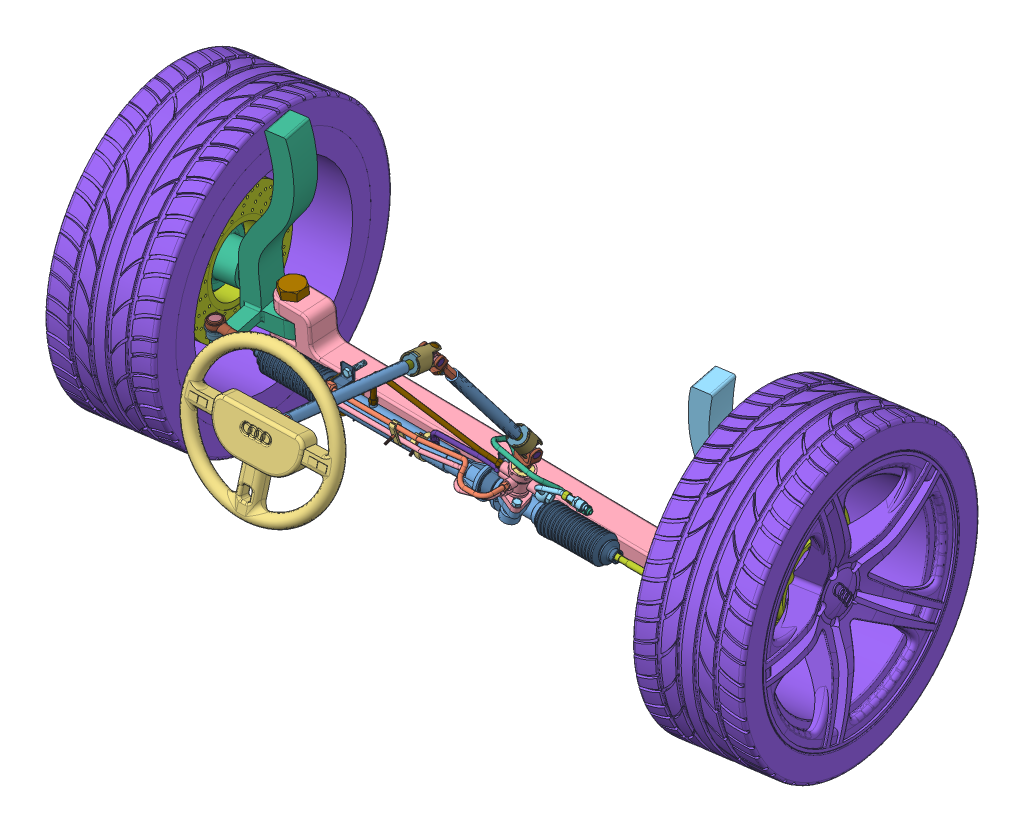
SolidWorks assembly 07, configuration Varsayılan. Lengths in mm.
Overall size (1849.54 1285.36 1549.53).
115 component instances, 65 part files, 142 mates.
Components (placement in the parent):
- 04-04-1: 04-04 [Varsayılan] at (-125.6681 -6.1583 231.0307) size (234.82 71.44 100.51)
- 04-02-1: 04-02 [Varsayılan] at (209.0718 -6.1583 231.0307) x (0 -1 0) z (-1 0 0) size (38 38 598)
- 04-03-1: 04-03 [Varsayılan] at (38.6922 -33.6461 251.0307) x (-0.603132 0.16779 0.779794) z (-0.75128 0.208941 -0.626037) size (25.52 151.51 25.52)
- 04-01-1: 04-01 [Varsayılan] at (50.1654 -6.1583 196.9106) x (0 0 1) z (-1 0 0) size (4.12 38.49 38.49)
- 04-05-1: 04-05 [Varsayılan] at (50.1654 -6.1583 220.9669) x (0 0 1) z (-1 0 0) size (15.7 26.77 26.77)
- 04-06-1: 04-06 [Varsayılan] at (50.1654 -6.1583 203.9669) x (-1 0 0) z (0 0 -1) size (18.46 18.46 19.47)
- 04-07-1: 04-07 [Varsayılan] at (50.1654 -6.1583 223.256) x (0 0 1) z (-1 0 0) size (13.68 21.45 8.13)
- 04-08-1: 04-08 [Varsayılan] at (50.1654 -6.1583 218.4607) x (0 1 0) z (-1 0 0) size (28.57 26.12 28.57)
- 05-14-1: 05-14 [Varsayılan] at (37.0194 -39.6612 251.0307) x (0.963448 -0.267897 0) z (0 0 1) size (30.59 16.59 30.59)
- 05-15-1: 05-15 [Varsayılan] at (41.4642 -23.6793 251.0307) x (0.963434 -0.267944 0) z (0 0 1) size (27.84 7.6 27.84)
- 05-21-1: 05-21 [Varsayılan] at (38.6909 -33.6508 251.0307) x (0.928206 -0.258147 -0.267944) z (0.267944 0.963434 0) size (19.84 10.08 10.35)
- 05-09-1: 05-09 [Varsayılan] at (52.7201 16.7932 251.0307) x (0.963434 -0.267944 0) z (0 0 1) size (31.93 8.54 31.93)
- 05-24-1: 05-24 [Varsayılan] at (55.0081 25.02 251.0307) x (0.963434 -0.267944 0) z (0 0 1) size (34.48 1.46 34.48)
- 05-19-1: 05-19 [Varsayılan] at (66.8414 67.5685 251.0307) x (0.963434 -0.267944 0) z (0 0 1) size (24.62 1.21 24.62)
- 05-10-1: 05-10 [Varsayılan] at (57.7931 35.0339 251.0307) x (0.959223 -0.266824 -0.093253) z (0.089843 -0.024987 0.995642) size (34.48 33.93 34.48)
- 05-11-1: 05-11 [Varsayılan] at (60.4905 44.7327 251.0307) x (0.963421 -0.267991 0) z (0 0 1) size (34.47 2.04 34.47)
- 05-11-2: 05-11 [Varsayılan] at (62.3958 51.5835 251.0307) x (0.963421 -0.267991 0) z (0 0 1) size (34.47 2.04 34.47)
- 05-11-3: 05-11 [Varsayılan] at (64.317 58.4914 251.0307) x (0.963421 -0.267991 0) z (0 0 1) size (34.47 2.04 34.47)
- 05-11-4: 05-11 [Varsayılan] at (66.126 64.9963 251.0307) x (0.963421 -0.267991 0) z (0 0 1) size (34.47 2.04 34.47)
- 05-12-1: 05-12 [Varsayılan] at (67.6163 70.3549 251.0307) x (0.92973 -0.25852 0.26224) z (-0.252651 0.070266 0.965003) size (31.17 6.94 31.17)
- 05-13-1: 05-13 [Varsayılan] at (69.4753 77.0389 251.0307) x (0.963448 -0.267897 0) z (0 0 1) size (29.11 4.72 29.11)
- 05-16-1: 05-16 [Varsayılan] at (67.6164 70.3551 251.0307) x (0.963448 -0.267897 0) z (0 0 1) size (40.01 14.09 40.01)
- 05-22-3: 05-22 [Varsayılan] at (69.4711 77.0238 251.0307) x (0.963434 -0.267944 0) z (0 0 1) size (37.74 2.78 37.74)
- 05-18-1: 05-18 [Varsayılan] at (71.3908 83.9265 251.0307) x (0.96127 -0.267342 0.066993) z (-0.064543 0.01795 0.997753) size (40.8 2.9 40.8)
- 05-25-1: 05-25 [Varsayılan] at (57.2884 33.5525 251.0071) x (0.003637 -0.001047 -0.999993) z (0.963428 -0.267942 0.003784) size (68.03 67.23 77.18)
- formed hex screw_am-1: formed hex screw_am [B18.2.3.2M - Formed hex screw, M10 x 1.5 x 25 --25WS] at (82.3436 33.466 275.1353) x (-0.267944 -0.963434 0) z (0 0 1) size (31.63 18.48 16)
- formed hex screw_am-2: formed hex screw_am [B18.2.3.2M - Formed hex screw, M10 x 1.5 x 25 --25WS] at (36.0727 46.3346 226.9262) x (-0.267944 -0.963434 0) z (0 0 1) size (31.63 18.48 16)
- ROT MİLİ-1: ROT MİLİ [Varsayılan] at (-398.6897 77.9473 255.0381) x (1 0 0) z (0 0.086009 -0.996294) size (284.47 41.76 37.89)
  - 02-02-2: 02-02 [Varsayılan] at (3.7615 85.8588 16.6847) size (48.52 36 36)
  - 02-03-3: 02-03 [Varsayılan] at (0.4735 85.8588 16.6847) x (-1 0 0) z (0 0.000479 1) size (257.66 24 24)
  - 02-01-2: 02-01 [Varsayılan] at (2.815 90.0301 15.9062) x (0.295289 -0.871295 0.391981) z (-0.068342 0.389963 0.918291) size (28 21.64 28)
- ROT MİLİ-2: ROT MİLİ [Varsayılan] at (218.8333 -67.283 293.5918) x (-1 0 0) z (0 -0.568825 -0.822459) size (284.47 41.76 37.89)
  - 02-02-2: 02-02 [Varsayılan] at (3.7615 85.8588 16.6847) size (48.52 36 36)
  - 02-03-3: 02-03 [Varsayılan] at (0.4735 85.8588 16.6847) x (-1 0 0) z (0 0.000479 1) size (257.66 24 24)
  - 02-01-2: 02-01 [Varsayılan] at (2.815 90.0301 15.9062) x (0.295289 -0.871295 0.391981) z (-0.068342 0.389963 0.918291) size (28 21.64 28)
- 05-31-1: 05-31 [Varsayılan] at (-390.0863 -6.1583 231.0307) x (0 0.999978 0.006566) z (0 0.006566 -0.999978) size (59.07 38.45 68.81)
- 05-02-1: 05-02 [Varsayılan] at (-409.0863 -6.1583 231.0307) x (-1 0 0) z (0 -0.999688 0.024965) size (174.75 66.11 66.11)
- 05-02-2: 05-02 [Varsayılan] at (105.6183 -6.1583 231.0307) size (174.75 66.11 66.11)
- ROT BAŞI-1: ROT BAŞI [Varsayılan] at (-649.4435 -11.5817 321.1285) x (1 0 0) z (0 0.087156 -0.996195) size (99.29 68.51 54.56)
  - 03-01-1: 03-01 [Default] at (-37.7726 9.1069 90.2276) size (90.23 26.88 54.56)
  - 03-02-1: 03-02 [Varsayılan] at (-32.6694 53.6205 89.5242) x (0 -1 0) z (0.136534 0 0.990635) size (58.89 20 20)
  - 03-03-1: 03-03 [Varsayılan] at (-37.7726 -12.3176 90.2276) x (0.135044 0.003215 -0.990834) z (0.99084 0 0.135044) size (26.35 4.4 26.35)
  - 03-04-1: 03-04 [Varsayılan] at (-37.7726 28.686 90.2276) x (0.880691 0 -0.473691) z (0.473691 0 0.880691) size (39.96 25.57 39.96)
  - 03-05-1: 03-05 [Varsayılan] at (-37.7726 -9.866 90.2276) size (25.83 14.98 25.83)
- ROT BAŞI-2: ROT BAŞI [Varsayılan] at (469.5871 4.146 141.36) x (-1 0 0) z (0 -0.087156 0.996195) size (99.29 68.51 54.56)
  - 03-01-1: 03-01 [Default] at (-37.7726 9.1069 90.2276) size (90.23 26.88 54.56)
  - 03-02-1: 03-02 [Varsayılan] at (-32.6694 53.6205 89.5242) x (0 -1 0) z (0.136534 0 0.990635) size (58.89 20 20)
  - 03-03-1: 03-03 [Varsayılan] at (-37.7726 -12.3176 90.2276) x (0.135044 0.003215 -0.990834) z (0.99084 0 0.135044) size (26.35 4.4 26.35)
  - 03-04-1: 03-04 [Varsayılan] at (-37.7726 28.686 90.2276) x (0.880691 0 -0.473691) z (0.473691 0 0.880691) size (39.96 25.57 39.96)
  - 03-05-1: 03-05 [Varsayılan] at (-37.7726 -9.866 90.2276) size (25.83 14.98 25.83)
- 05-28-1: 05-28 [Varsayılan] at (-1.0263 -6.1583 231.0307) x (0 -0.759317 -0.650721) z (-1 0 0) size (54.92 54.94 38.56)
- 05-05-3: 05-05 [Varsayılan] at (-153.627 16.7021 236.5228) x (-0.999618 0.007048 -0.026719) z (0.027616 0.221471 -0.974776) size (188.63 58.73 20.5)
- 05-06-2: 05-06 [Varsayılan] at (-308.371 55.2453 229.576) x (-0.999565 0.002273 -0.029406) z (0.029339 -0.025305 -0.999249) size (348.36 70.43 41.18)
- 05-03-3: 05-03 [Varsayılan] at (-414.0863 -6.1583 231.0307) size (295 48.35 43.5)
- 05-33-1: 05-33 [Default] at (-156.8797 44.8002 297.1129) x (-1 0 0) z (0 0.302472 -0.953158) size (421.56 52.06 61.28)
- 05-01-1: 05-01 [Varsayılan] at (-173.5526 -6.1583 231.0307) x (-1 0 0) z (0 0.360562 -0.932735) size (14 137.7 76.92)
- 05-04-1: 05-04 [Varsayılan] at (-390.9146 51.2479 300.523) x (-0.991921 0.112405 0.058801) z (0.000453 0.46666 -0.884437) size (456.96 84.72 60.1)
- 05-08-1: 05-08 [Varsayılan] at (237.637 92.2948 265.4276) x (-0.997325 0.072053 -0.012308) z (-0.043043 -0.714977 -0.697822) size (140.05 46.48 89.04)
- 05-07-1: 05-07 [Varsayılan] at (228.5019 70.3353 246.6946) x (-0.999175 0.040461 0.003581) z (-0.026401 -0.579908 -0.814254) size (231 45.96 100.61)
- formed hex screw_am-3: formed hex screw_am [B18.2.3.2M - Formed hex screw, M12 x 1.75 x 25 --25WS] at (123.6594 37.5337 232.8376) x (-0.948079 0.263674 0.177825) z (-0.177825 -0.903067 0.390959) size (32.76 20.78 18)
- 05-27-1: 05-27 [Varsayılan] at (186.4406 76.9952 250.3773) x (0.044464 0.751851 0.657832) z (0.9987 -0.049876 -0.0105) size (45.68 8 10)
- 05-27-2: 05-27 [Varsayılan] at (196.4276 76.4964 250.2723) x (0.044464 0.751851 0.657832) z (-0.9987 0.049876 0.0105) size (45.68 8 10)
- hex screw_am-2: hex screw_am [B18.6.7M - M5 x 0.8 x 10 Indented HHMS --10S] at (191.9929 87.5632 252.0852) x (-0.024915 -0.657444 0.753091) z (-0.753091 0.507767 0.418362) size (13.8 9.24 8)
- prevailing torque hex nut_am-2: prevailing torque hex nut_am [AM-M5-S] at (191.6665 78.9507 261.9507) x (0.999646 -0.009344 0.024915) z (-0.024915 -0.657444 0.753091) size (8 9.81 5.3)
- 05-29-1: 05-29 [Default] at (-12.3188 -6.1583 205.6444) x (0 1 0) z (0 0 -1) size (108.96 30.28 55.85)
- 05-29-3: 05-29 [Default] at (-390.1285 -6.1115 206.1523) x (0 0.999914 0.013132) z (0 0.013132 -0.999914) size (108.96 30.28 55.85)
- formed hex screw_am-4: formed hex screw_am [B18.2.3.2M - Formed hex screw, M10 x 1.5 x 40 --26WS] at (-390.1268 33.0747 215.2976) x (0 0.013132 -0.999914) z (0.935126 0.354284 0.004653) size (46.63 18.48 16)
- formed hex screw_am-5: formed hex screw_am [B18.2.3.2M - Formed hex screw, M10 x 1.5 x 40 --26WS] at (-390.1268 -45.812 214.2616) x (0 0.013132 -0.999914) z (0.970956 -0.239236 -0.003142) size (46.63 18.48 16)
- formed hex screw_am-6: formed hex screw_am [B18.2.3.2M - Formed hex screw, M10 x 1.5 x 40 --26WS] at (-12.3171 -45.7489 214.2744) x (0 0 -1) z (0.991782 -0.12794 0) size (46.63 18.48 16)
- formed hex screw_am-7: formed hex screw_am [B18.2.3.2M - Formed hex screw, M10 x 1.5 x 40 --26WS] at (-12.3171 33.1445 213.7744) x (0 0 -1) z (0.999706 0.024251 0) size (46.63 18.48 16)
- UNIVERSAL MAFSAL-1: UNIVERSAL MAFSAL [Varsayılan] at (141.0332 165.171 256.4603) x (0.950533 -0.264356 0.163103) z (-0.267944 -0.963434 0) size (48.16 92.97 129.43)
  - 01-01-1: 01-01 [Varsayılan] at (-45.6055 2.036 86.4549) size (47 34.99 57.64)
  - 01-02-1: 01-02 [Varsayılan] at (-45.0363 8.2494 31.8587) x (-0.051046 -0.624854 0.779071) z (0 -0.780088 -0.62567) size (70.3 43.23 43.34)
  - 01-03-1: 01-03 [Varsayılan] at (-51.6055 -0.2661 32.8861) x (1 0 0) z (0 -0.62567 0.780088) size (36 31 16)
  - 01-04-1: 01-04 [Varsayılan] at (-42.5986 38.09 -5.3467) x (-0.998696 0.031938 -0.03982) z (-0.051046 -0.624854 0.779071) size (33.8 41.3 6)
  - 01-05-1: 01-05 [Varsayılan] at (-42.9049 34.3409 -0.6723) x (0.998255 -0.008733 0.058403) z (0.02969 -0.780692 -0.62421) size (32.2 29.4 32.2)
  - 01-06-1: 01-06 [Varsayılan] at (-44.4056 15.9701 22.2324) x (0.051046 0.624854 -0.779071) z (0.993628 0.046715 0.102572) size (75.7 17.29 17.32)
  - 01-07-1: 01-07 [Varsayılan] at (-25.3055 1.2861 40.5406) x (0 0 -1) z (1 0 0) size (16 16 15)
  - 01-08-1: 01-08 [Varsayılan] at (-45.6055 -12.5995 29.4036) x (0.792707 0.38141 -0.475544) z (0 -0.780088 -0.62567) size (16 16 15)
  - 01-07-2: 01-07 [Varsayılan] at (-65.9055 1.2861 40.5406) x (0 -0.633294 0.773912) z (-1 0 0) size (16 16 15)
  - 01-08-2: 01-08 [Varsayılan] at (-45.6055 15.1716 51.6775) x (0.990366 0.086641 -0.108024) z (0 0.780088 0.62567) size (16 16 15)
  - formed hex screw_am-1: formed hex screw_am [B18.2.3.2M - Formed hex screw, M6 x 1.0 x 35 --18WS] at (-62.5055 12.536 76.9549) x (1 0 0) z (0 0.052048 -0.998645) size (39.15 11.55 10)
  - prevailing torque hex nut_am-1: prevailing torque hex nut_am [AM-M6-S] at (-26.1555 12.536 76.9549) x (0 0.889289 0.457347) z (1 0 0) size (10.79 11.55 6.7)
- SHAFT 1-1: SHAFT 1 [Varsayılan] at (102.4 214.0531 312.2723) x (0.979633 -0.04367 -0.195992) z (0.15908 0.764397 0.624813) size (24 24 322.5)
- SHAFT 2-1: SHAFT 2 [Varsayılan] at (126.2619 328.7127 405.9942) x (-0.986743 0.10251 0.125818) z (0.15908 0.764397 0.624813) size (19 19 232)
- UNIVERSAL MAFSAL-2: UNIVERSAL MAFSAL [Varsayılan] at (218.869 550.0843 590.8605) x (0.981176 -0.192592 -0.014194) z (-0.15908 -0.764397 -0.624813) size (48.16 92.97 129.43)
  - 01-01-1: 01-01 [Varsayılan] at (-45.6055 2.036 86.4549) size (47 34.99 57.64)
  - 01-02-1: 01-02 [Varsayılan] at (-45.0363 8.2494 31.8587) x (-0.051046 -0.624854 0.779071) z (0 -0.780088 -0.62567) size (70.3 43.23 43.34)
  - 01-03-1: 01-03 [Varsayılan] at (-51.6055 -0.2661 32.8861) x (1 0 0) z (0 -0.62567 0.780088) size (36 31 16)
  - 01-04-1: 01-04 [Varsayılan] at (-42.5986 38.09 -5.3467) x (-0.998696 0.031938 -0.03982) z (-0.051046 -0.624854 0.779071) size (33.8 41.3 6)
  - 01-05-1: 01-05 [Varsayılan] at (-42.9049 34.3409 -0.6723) x (0.998255 -0.008733 0.058403) z (0.02969 -0.780692 -0.62421) size (32.2 29.4 32.2)
  - 01-06-1: 01-06 [Varsayılan] at (-44.4056 15.9701 22.2324) x (0.051046 0.624854 -0.779071) z (0.993628 0.046715 0.102572) size (75.7 17.29 17.32)
  - 01-07-1: 01-07 [Varsayılan] at (-25.3055 1.2861 40.5406) x (0 0 -1) z (1 0 0) size (16 16 15)
  - 01-08-1: 01-08 [Varsayılan] at (-45.6055 -12.5995 29.4036) x (0.792707 0.38141 -0.475544) z (0 -0.780088 -0.62567) size (16 16 15)
  - 01-07-2: 01-07 [Varsayılan] at (-65.9055 1.2861 40.5406) x (0 -0.633294 0.773912) z (-1 0 0) size (16 16 15)
  - 01-08-2: 01-08 [Varsayılan] at (-45.6055 15.1716 51.6775) x (0.990366 0.086641 -0.108024) z (0 0.780088 0.62567) size (16 16 15)
  - formed hex screw_am-1: formed hex screw_am [B18.2.3.2M - Formed hex screw, M6 x 1.0 x 35 --18WS] at (-62.5055 12.536 76.9549) x (1 0 0) z (0 0.052048 -0.998645) size (39.15 11.55 10)
  - prevailing torque hex nut_am-1: prevailing torque hex nut_am [AM-M6-S] at (-26.1555 12.536 76.9549) x (0 0.889289 0.457347) z (1 0 0) size (10.79 11.55 6.7)
- SHAFT 1-2: SHAFT 1 [Varsayılan] at (178.0086 547.047 663.7863) x (0.966904 0.207955 -0.147823) z (0.105608 0.201209 0.973839) size (24 24 322.5)
- SHAFT 2-2: SHAFT 2 [Varsayılan] at (191.7377 573.2042 790.3853) x (-0.993361 0.06628 0.094031) z (0.105608 0.201209 0.973839) size (19 19 232)
- direksiyon-1: direksiyon [Varsayılan] at (216.7667 620.8908 1021.1848) x (-0.993361 0.06628 0.094031) z (0.105608 0.201209 0.973839) size (350 350 50.57)
- ÖN DÜZEN-1: ÖN DÜZEN [Varsayılan] at (-260.8263 1115.8453 259.3364) x (-0.999881 0.001392 -0.015371) z (-0.000148 -0.996747 -0.080594) size (1834.03 1010.52 929.37)
  - DİNGİL-1: DİNGİL [Varsayılan] at (-152.2952 42.0235 1230.14) size (1171.64 67 117)
  - Tekerlek porya-bağlantı kolları  R-1: Tekerlek porya-bağlantı kolları  R [Varsayılan] at (-732.3489 82.2489 1097.7024) x (-0.988638 0.150316 0) z (0.150316 0.988638 0) size (231.48 449.46 221.1)
  - Tekerlek porya-bağlantı kolları L-1: Tekerlek porya-bağlantı kolları L [Varsayılan] at (427.7584 68.798 1097.7024) x (0.988638 -0.150316 0) z (-0.150316 -0.988638 0) size (231.48 449.46 221.1)
  - Fren diski-1: Fren diski [Varsayılan] at (509.8767 56.3125 1097.7024) x (-0.084581 -0.556299 0.826667) z (0.124261 0.817274 0.562692) size (303 56.33 303)
  - Tekerlek-1: Tekerlek [Varsayılan] at (-277.6343 176.0481 1097.7024) x (-0.084581 -0.556299 0.826667) z (0.124261 0.817274 0.562692) size (668.92 273.92 668.92)
  - Fren diski-2: Fren diski [Varsayılan] at (-814.4672 94.7344 1097.7024) x (-0.080555 -0.529817 -0.844277) z (0.126908 0.834685 -0.535906) size (303 56.33 303)
  - Tekerlek-2: Tekerlek [Varsayılan] at (-26.9562 -25.0012 1097.7024) x (-0.080555 -0.529817 -0.844277) z (0.126908 0.834685 -0.535906) size (668.92 273.92 668.92)
  - heavy hex bolt_am-2: heavy hex bolt_am [B18.2.3.6M - Heavy hex bolt M30 x 3.5 x 140 --72S] at (383.5248 75.5235 1093.39) x (0 0 1) z (-1 0 0) size (159.75 57.74 50)
  - hex nut heavy_am-2: hex nut heavy_am [B18.2.4.6M - Heavy hex nut,  M30 x 3.5 --W-S] at (383.5248 75.5235 1260.84) size (50 57.74 30.7)
  - heavy hex bolt_am-3: heavy hex bolt_am [B18.2.3.6M - Heavy hex bolt M30 x 3.5 x 140 --72S] at (-688.1152 75.5235 1093.39) x (0 0 1) z (-1 0 0) size (159.75 57.74 50)
  - hex nut heavy_am-3: hex nut heavy_am [B18.2.4.6M - Heavy hex nut,  M30 x 3.5 --W-S] at (-688.1152 75.5235 1260.84) size (50 57.74 30.7)
- 05-30-1: 05-30 [B18.2.3.2M - Formed hex screw, M5 x 0.8 x 40 --16WS] at (-179.5526 27.5361 241.8952) x (0 -0.741989 0.670412) z (-0.831659 0.372271 0.412016) size (43.65 9.24 8)
- 05-30-2: 05-30 [B18.2.3.2M - Formed hex screw, M5 x 0.8 x 40 --16WS] at (-179.5526 63.0693 290.0383) x (0 -0.309906 0.950767) z (-0.960688 -0.26396 -0.086039) size (43.65 9.24 8)
Mates (geometry in assembly coordinates):
- Eş Merkezli1: concentric aligned: cylinder of 04-04-1 through (-165.266 -6.1583 231.0307) axis (1 0 0) radius 14; cylinder of 04-02-1 through (-388.9282 -6.1583 231.0307) axis (1 0 0) radius 11.5
- Eş Merkezli2: concentric anti-aligned: cylinder of 04-04-1 through (54.1024 21.7633 251.0307) axis (0.267944 0.963434 0) radius 12.4576; line of 04-03-1 through (79.2895 112.3275 251.0307) axis (-0.267944 -0.963434 0)
- Teğet1: tangent aligned: plane of 04-04-1 through (55.5026 -19.6951 251.0307) normal (-0.267944 -0.963434 0); cone of 04-03-1 through (43.5006 -16.3571 251.0307) axis (-0.267944 -0.963434 0)
- Paralel1: parallel: plane of 04-02-1 through (46.1449 10.9835 238.0307) normal (0 0 1); line of 04-03-1 through (79.2895 112.3275 251.0307) axis (-0.267944 -0.963434 0)
- RackPinionMate1: rack pinion = 20 mm: line of 04-02-1 through (7.4299 -15.2825 238.0307) axis (-1 0 0); circle of 04-03-1
- Uzaklığı Sınırla1: limit distance = 45.2601 mm anti-aligned: plane of 04-04-1 through (-125.6681 11.3406 231.0307) normal (-1 0 0); plane of 04-02-1 through (-170.9282 -6.1583 250.0307) normal (1 0 0)
- Eş Merkezli3: concentric anti-aligned: cylinder of 04-05-1 through (50.1654 -6.1583 220.9669) axis (0 0 -1) radius 3.705; cylinder of 04-07-1 through (50.1654 -6.1583 223.256) axis (0 0 1) radius 3.7071
- Eş Merkezli4: concentric: sphere of 04-05-1; unknown of 04-07-1
- Eş Merkezli5: concentric anti-aligned: circle of 04-06-1; cylinder of 04-07-1 through (50.1654 -6.1583 223.256) axis (0 0 1) radius 3.7071
- Çakışık1: coincident anti-aligned: plane of 04-05-1 through (59.8031 -6.1583 220.9669) normal (0 0 -1); plane of 04-06-1 through (40.4527 -15.387 220.9669) normal (0 0 1)
- Eş Merkezli6: concentric anti-aligned: circle of 04-06-1; cylinder of 04-08-1 through (50.1654 -6.1583 199.3607) axis (0 0 1) radius 14.285
- Çakışık2: coincident anti-aligned: plane of 04-05-1 through (63.3694 -6.1583 218.4607) normal (0 0 -1); plane of 04-08-1 through (50.1654 -6.1583 218.4607) normal (0 0 1)
- Eş Merkezli7: concentric anti-aligned: cylinder of 04-04-1 through (50.1654 -6.1583 285.0814) axis (0 0 -1) radius 14; cylinder of 04-08-1 through (50.1654 -6.1583 199.3607) axis (0 0 1) radius 14.285
- Çakışık3: coincident anti-aligned: plane of 04-04-1 through (50.1654 -6.1583 201.0307) normal (0 0 -1); circle of 04-08-1
- Eş Merkezli8: concentric anti-aligned: cylinder of 04-04-1 through (50.1654 -6.1583 201.0307) axis (0 0 1) radius 18.85; cylinder of 04-01-1 through (50.1654 -6.1583 196.9106) axis (0 0 -1) radius 13.3852
- Çakışık4: coincident anti-aligned: plane of 04-04-1 through (50.1654 -6.1583 201.0307) normal (0 0 -1); plane of 04-01-1 through (63.5506 -6.1583 201.0307) normal (0 0 1)
- Eş Merkezli9: concentric anti-aligned: cylinder of 04-04-1 through (54.1024 21.7633 251.0307) axis (0.267944 0.963434 0) radius 15.0252; cylinder of 05-15-1 through (43.5005 -16.3572 251.0307) axis (-0.267944 -0.963434 0) radius 13.92
- Çakışık5: coincident anti-aligned: plane of 04-04-1 through (55.5026 -19.6951 251.0307) normal (-0.267944 -0.963434 0); plane of 05-15-1 through (43.5005 -16.3572 251.0307) normal (0.267944 0.963434 0)
- Eş Merkezli10: concentric aligned: cone of 04-03-1 through (38.6923 -33.6459 251.0307) axis (0.267944 0.963434 0); cylinder of 05-21-1 through (38.6909 -33.6508 251.0307) axis (0.267944 0.963434 0) radius 4.26
- Çakışık6: coincident anti-aligned: plane of 05-15-1 through (41.4642 -23.6793 251.0307) normal (-0.267944 -0.963434 0); plane of 05-21-1 through (41.4642 -23.6793 251.0307) normal (0.267944 0.963434 0)
- Eş Merkezli11: concentric aligned: cylinder of 04-04-1 through (54.1024 21.7633 251.0307) axis (0.267944 0.963434 0) radius 15.0252; cone of 05-14-1 through (39.1828 -31.8821 251.0307) axis (0.267944 0.963434 0)
- Teğet2: tangent aligned: cone of 05-14-1 through (41.4644 -23.6786 251.0307) axis (-0.267944 -0.963434 0); plane of 05-15-1 through (41.4642 -23.6793 251.0307) normal (-0.267944 -0.963434 0)
- Çakışık7: coincident: circle of 04-03-1; cylinder of 05-09-1 through (52.7203 16.7938 251.0307) axis (-0.267944 -0.963434 0) radius 1570.6986
- Eş Merkezli13: concentric anti-aligned: cylinder of 04-03-1 through (38.6922 -33.6461 251.0307) axis (-0.267944 -0.963434 0) radius 12.7592; cone of 05-24-1 through (55.3984 26.4235 251.0307) axis (0.267944 0.963434 0)
- Çakışık8: coincident aligned: cone of 05-09-1 through (55.008 25.0198 251.0307) axis (-0.267944 -0.963434 0); cone of 05-24-1 through (55.0081 25.02 251.0307) axis (-0.267944 -0.963434 0)
- Eş Merkezli14: concentric anti-aligned: cylinder of 04-03-1 through (67.1664 68.737 251.0307) axis (0.267944 0.963434 0) radius 0.0489; circle of 05-19-1
- Teğet4: tangent aligned: cone of 04-03-1 through (66.8415 67.569 251.0307) axis (-0.267944 -0.963434 0); plane of 05-19-1 through (66.8414 67.5685 251.0307) normal (-0.267944 -0.963434 0)
- Eş Merkezli15: concentric anti-aligned: cone of 04-03-1 through (67.1664 68.737 251.0307) axis (0.267944 0.963434 0); cone of 05-10-1 through (58.0414 35.9269 251.0307) axis (-0.267944 -0.963434 0)
- Teğet5: tangent aligned: plane of 05-19-1 through (66.8414 67.5685 251.0307) normal (-0.267944 -0.963434 0); cone of 05-10-1 through (66.8415 67.569 251.0307) axis (-0.267944 -0.963434 0)
- Eş Merkezli17: concentric aligned: cone of 05-10-1 through (60.4905 44.7327 251.0307) axis (0.267944 0.963434 0); cone of 05-11-1 through (61.036 46.6943 251.0307) axis (0.267944 0.963434 0)
- Çakışık10: coincident: circle of 05-10-1; cylinder of 05-11-1 through (60.4905 44.7327 251.0307) axis (-0.267944 -0.963434 0) radius 1570.7474
- Eş Merkezli18: concentric aligned: cone of 05-10-1 through (62.3958 51.5835 251.0307) axis (0.267944 0.963434 0); cone of 05-11-2 through (62.9413 53.5452 251.0307) axis (0.267944 0.963434 0)
- Çakışık11: coincident: circle of 05-10-1; cylinder of 05-11-2 through (62.3958 51.5835 251.0307) axis (-0.267944 -0.963434 0) radius 1570.7474
- Eş Merkezli19: concentric aligned: cone of 05-10-1 through (64.317 58.4914 251.0307) axis (0.267944 0.963434 0); cone of 05-11-3 through (64.8625 60.4531 251.0307) axis (0.267944 0.963434 0)
- Çakışık12: coincident: circle of 05-10-1; cylinder of 05-11-3 through (64.317 58.4914 251.0307) axis (-0.267944 -0.963434 0) radius 1570.7474
- Eş Merkezli20: concentric aligned: cone of 05-10-1 through (66.126 64.9963 251.0307) axis (0.267944 0.963434 0); cone of 05-11-4 through (66.6716 66.9579 251.0307) axis (0.267944 0.963434 0)
- Çakışık13: coincident: circle of 05-10-1; cylinder of 05-11-4 through (66.126 64.9963 251.0307) axis (-0.267944 -0.963434 0) radius 1570.7474
- Eş Merkezli22: concentric aligned: cone of 04-03-1 through (67.1664 68.737 251.0307) axis (0.267944 0.963434 0); cone of 05-12-1 through (69.4753 77.0389 251.0307) axis (0.267944 0.963434 0)
- Uzaklık1: distance = 2.73 mm aligned: cone of 05-12-1 through (67.6163 70.3549 251.0307) axis (-0.267944 -0.963434 0); cone of 05-10-1 through (66.8849 67.725 251.0307) axis (-0.267944 -0.963434 0)
- Eş Merkezli23: concentric aligned: cone of 04-03-1 through (67.1664 68.737 251.0307) axis (0.267944 0.963434 0); cone of 05-13-1 through (70.7393 81.5839 251.0307) axis (0.267944 0.963434 0)
- Çakışık14: coincident aligned: cone of 05-12-1 through (69.4753 77.0392 251.0307) axis (-0.267944 -0.963434 0); cone of 05-13-1 through (69.4753 77.0389 251.0307) axis (-0.267944 -0.963434 0)
- Eş Merkezli24: concentric aligned: cone of 05-12-1 through (67.6164 70.3551 251.0307) axis (0.267944 0.963434 0); cone of 05-16-1 through (67.6165 70.3553 251.0307) axis (0.267944 0.963434 0)
- Çakışık15: coincident aligned: cone of 05-12-1 through (67.6163 70.3549 251.0307) axis (-0.267944 -0.963434 0); cone of 05-16-1 through (67.6164 70.3551 251.0307) axis (-0.267944 -0.963434 0)
- Eş Merkezli25: concentric anti-aligned: cone of 05-16-1 through (69.4711 77.0238 251.0307) axis (0.267944 0.963434 0); cylinder of 05-22-3 through (70.216 79.7022 251.0307) axis (-0.267944 -0.963434 0) radius 18.87
- Çakışık16: coincident aligned: circle of 05-16-1; plane of 05-22-3 through (69.4711 77.0238 251.0307) normal (-0.267944 -0.963434 0)
- Eş Merkezli26: concentric anti-aligned: cone of 04-03-1 through (67.1664 68.737 251.0307) axis (0.267944 0.963434 0); cylinder of 05-18-1 through (76.4549 102.1354 251.0307) axis (-0.267944 -0.963434 0) radius 9.8
- Teğet6: tangent aligned: cone of 05-16-1 through (71.391 83.9274 251.0307) axis (-0.267944 -0.963434 0); plane of 05-18-1 through (71.3908 83.9265 251.0307) normal (-0.267944 -0.963434 0)
- Eş Merkezli27: concentric aligned: cylinder of 04-04-1 through (47.6487 -91.2848 275.1353) axis (0.267944 0.963434 0) radius 5.0797; cylinder of 05-25-1 through (77.2955 15.3149 275.1353) axis (0.267944 0.963434 0) radius 4.95
- Eş Merkezli28: concentric aligned: cylinder of 04-04-1 through (1.3778 -78.4162 226.9262) axis (0.267944 0.963434 0) radius 4.95; cylinder of 05-25-1 through (31.0246 28.1834 226.9262) axis (0.267944 0.963434 0) radius 5.0797
- Çakışık17: coincident anti-aligned: plane of 04-04-1 through (81.3463 14.1883 251.0307) normal (0.267944 0.963434 0); plane of 05-25-1 through (54.0168 21.789 251.0071) normal (-0.267944 -0.963434 0)
- Eş Merkezli291: concentric aligned: cylinder of 05-25-1 through (77.2955 15.3149 275.1353) axis (0.267944 0.963434 0) radius 4.95; cylinder of formed hex screw_am-1 through (82.3436 33.466 275.1353) axis (0.267944 0.963434 0) radius 5
- Çakışık181: coincident anti-aligned: plane of 05-25-1 through (57.2884 33.5525 251.0071) normal (0.267944 0.963434 0); plane of formed hex screw_am-1 through (89.4669 24.6032 275.1353) normal (-0.267944 -0.963434 0)
- Eş Merkezli301: concentric aligned: cylinder of 05-25-1 through (31.0246 28.1834 226.9262) axis (0.267944 0.963434 0) radius 5.0797; cylinder of formed hex screw_am-2 through (36.0727 46.3346 226.9262) axis (0.267944 0.963434 0) radius 5
- Çakışık191: coincident anti-aligned: plane of 05-25-1 through (57.2884 33.5525 251.0071) normal (0.267944 0.963434 0); plane of formed hex screw_am-2 through (43.196 37.4718 226.9262) normal (-0.267944 -0.963434 0)
- Eş Merkezli32: concentric anti-aligned: cylinder of 04-02-1 through (-388.9282 -6.1583 231.0307) axis (1 0 0) radius 11.5; cylinder of ROT MİLİ-1/02-02-2 through (-395.0817 -6.1583 231.0307) axis (-1 0 0) radius 18
- Çakışık20: coincident anti-aligned: plane of 04-02-1 through (-388.9282 -6.1583 231.0307) normal (-1 0 0); plane of ROT MİLİ-1/02-02-2 through (-388.9282 -6.1583 231.0307) normal (1 0 0)
- Eş Merkezli33: concentric aligned: cylinder of 04-02-1 through (-388.9282 -6.1583 231.0307) axis (1 0 0) radius 11.5; cylinder of ROT MİLİ-2/02-02-2 through (215.2253 -6.1583 231.0307) axis (1 0 0) radius 18
- Çakışık21: coincident anti-aligned: plane of 04-02-1 through (209.0718 -6.1583 231.0307) normal (1 0 0); plane of ROT MİLİ-2/02-02-2 through (209.0718 -6.1583 231.0307) normal (-1 0 0)
- Eş Merkezli36: concentric anti-aligned: cylinder of 04-02-1 through (-388.9282 -6.1583 231.0307) axis (1 0 0) radius 11.5; cylinder of 05-02-2 through (105.6183 -6.1583 231.0307) axis (-1 0 0) radius 11.6806
- Çakışık23: coincident anti-aligned: plane of 04-04-1 through (105.6183 12.6764 231.0307) normal (1 0 0); plane of 05-02-2 through (105.6183 19.7754 231.0307) normal (-1 0 0)
- Eş Merkezli37: concentric aligned: cylinder of ROT MİLİ-1/02-03-3 through (-409.2161 -6.1583 231.0307) axis (1 0 0) radius 5.0675; cylinder of ROT BAŞI-1/03-01-1 through (-651.9661 -6.1583 231.0307) axis (1 0 0) radius 9.5
- Çakışık24: coincident aligned: circle of ROT MİLİ-1/02-03-3; plane of ROT BAŞI-1/03-01-1 through (-615.2161 3.1472 222.1941) normal (1 0 0)
- Eş Merkezli38: concentric aligned: cylinder of ROT MİLİ-2/02-03-3 through (229.3597 -6.1583 231.0307) axis (-1 0 0) radius 6.5; cylinder of ROT BAŞI-2/03-01-1 through (472.1097 -6.1583 231.0307) axis (-1 0 0) radius 9.5
- Çakışık25: coincident aligned: circle of ROT MİLİ-2/02-03-3; plane of ROT BAŞI-2/03-01-1 through (435.3597 1.4714 241.349) normal (-1 0 0)
- Eş Merkezli39: concentric anti-aligned: cylinder of 04-04-1 through (-125.6681 -6.1583 231.0307) axis (-1 0 0) radius 21.75; cylinder of 05-28-1 through (-23.5863 -6.1583 231.0307) axis (1 0 0) radius 25.75
- Çakışık26: coincident anti-aligned: plane of 04-04-1 through (6.9737 26.3417 231.0307) normal (-1 0 0); plane of 05-28-1 through (6.9737 -6.1583 231.0307) normal (1 0 0)
- Eş Merkezli304: concentric anti-aligned: cylinder of 05-25-1 through (101.3768 36.6462 241.4658) axis (-0.949417 0.264046 0.169963) radius 5; cylinder of 05-05-3 through (21.6687 58.8141 255.7351) axis (0.949417 -0.264046 -0.169963) radius 7
- Çakışık194: coincident anti-aligned: plane of 05-25-1 through (21.5918 48.3269 253.9468) normal (-0.949417 0.264046 0.169963); plane of 05-05-3 through (26.0012 62.678 256.2827) normal (0.949417 -0.264046 -0.169963)
- Eş Merkezli305: concentric anti-aligned: cylinder of 05-25-1 through (105.7565 50.9201 243.7559) axis (-0.949417 0.264046 0.169963) radius 5; cylinder of 05-06-2 through (26.0484 73.088 258.0251) axis (0.949417 -0.264046 -0.169963) radius 7
- Çakışık195: coincident anti-aligned: plane of 05-25-1 through (21.5918 48.3269 253.9468) normal (-0.949417 0.264046 0.169963); plane of 05-06-2 through (30.1982 77.1184 257.2936) normal (0.949417 -0.264046 -0.169963)
- Eş Merkezli306: concentric anti-aligned: cylinder of 04-02-1 through (-388.9282 -6.1583 231.0307) axis (1 0 0) radius 11.5; cylinder of 05-03-3 through (-119.0863 -6.1583 231.0307) axis (-1 0 0) radius 21.75
- Çakışık196: coincident anti-aligned: plane of 04-04-1 through (-119.0863 12.8417 231.0307) normal (-1 0 0); plane of 05-03-3 through (-119.0863 -6.1583 231.0307) normal (1 0 0)
- Eş Merkezli307: concentric anti-aligned: cylinder of 05-31-1 through (-405.0863 -6.1583 231.0307) axis (1 0 0) radius 20.7084; cylinder of 05-03-3 through (-119.0863 -6.1583 231.0307) axis (-1 0 0) radius 21.75
- Eş Merkezli308: concentric anti-aligned: cylinder of 05-02-1 through (-409.0863 -6.1583 231.0307) axis (1 0 0) radius 25.6827; cylinder of 05-03-3 through (-119.0863 -6.1583 231.0307) axis (-1 0 0) radius 21.75
- Uzaklık2: distance = 5 mm aligned: plane of 05-03-3 through (-414.0863 -6.1583 231.0307) normal (-1 0 0); plane of 05-31-1 through (-409.0863 -6.1583 231.0307) normal (-1 0 0)
- Çakışık197: coincident anti-aligned: plane of 05-31-1 through (-409.0863 -6.1583 231.0307) normal (-1 0 0); plane of 05-02-1 through (-409.0863 -6.8058 205.105) normal (1 0 0)
- Kilitle1: lock: unknown of 05-05-3; unknown of 05-03-3
- Kilitle2: lock: unknown of 05-06-2; unknown of 05-03-3
- Eş Merkezli309: concentric anti-aligned: cylinder of 05-25-1 through (65.5394 62.2675 263.2963) axis (-0.003655 0.006527 0.999972) radius 5; cylinder of 05-33-1 through (65.3201 62.6591 323.2946) axis (0.003655 -0.006527 -0.999972) radius 4
- Çakışık198: coincident anti-aligned: plane of 05-25-1 through (60.6154 54.5186 283.3295) normal (-0.003655 0.006527 0.999972); plane of 05-33-1 through (65.4663 62.3981 283.2958) normal (0.003655 -0.006527 -0.999972)
- Eş Merkezli310: concentric anti-aligned: cylinder of 05-03-3 through (-119.0863 -6.1583 231.0307) axis (-1 0 0) radius 21.75; cylinder of 05-01-1 through (-185.5526 -6.1583 231.0307) axis (1 0 0) radius 21.7671
- Teğet7: tangent anti-aligned: cylinder of 05-33-1 through (-125.1716 75.9211 306.9887) axis (-1 0 0) radius 5; plane of 05-01-1 through (-172.5526 79.1244 302.774) normal (0 -0.309917 0.950763)
- Eş Merkezli312: concentric anti-aligned: cylinder of 05-25-1 through (55.8376 46.5086 263.3637) axis (-0.003655 0.006527 0.999972) radius 5; circle of 05-04-1
- Çakışık201: coincident anti-aligned: plane of 05-25-1 through (60.6154 54.5186 283.3295) normal (-0.003655 0.006527 0.999972); plane of 05-04-1 through (60.0822 49.1995 283.3622) normal (0.003655 -0.006527 -0.999972)
- Kilitle3: lock: unknown of 05-01-1; unknown of 05-04-1
- Eş Merkezli313: concentric aligned: cylinder of 05-25-1 through (18.9204 66.663 252.4828) axis (0.948079 -0.263674 -0.177825) radius 5; cylinder of 05-08-1 through (83.9328 48.5821 240.2888) axis (0.948079 -0.263674 -0.177825) radius 5
- Çakışık202: coincident anti-aligned: plane of 05-25-1 through (97.3407 44.8532 237.774) normal (0.948079 -0.263674 -0.177825); plane of 05-08-1 through (101.3663 42.9237 262.0976) normal (-0.948079 0.263674 0.177825)
- Eş Merkezli314: concentric anti-aligned: cylinder of 05-25-1 through (91.8203 46.3885 292.2446) axis (-0.66663 0.185399 -0.721963) radius 5; cylinder of 05-07-1 through (28.8333 63.9061 224.0295) axis (0.66663 -0.185399 0.721963) radius 3
- Çakışık203: coincident anti-aligned: plane of 05-25-1 through (40.3095 60.7144 222.006) normal (-0.66663 0.185399 -0.721963); plane of 05-07-1 through (29.8159 63.3842 232.381) normal (0.66663 -0.185399 0.721963)
- Eş Merkezli3151: concentric aligned: cylinder of 05-08-1 through (83.9328 48.5821 240.2888) axis (0.948079 -0.263674 -0.177825) radius 5; cylinder of formed hex screw_am-3 through (123.6594 37.5337 232.8376) axis (0.948079 -0.263674 -0.177825) radius 6
- Çakışık2041: coincident anti-aligned: plane of 05-08-1 through (120.4882 37.9933 258.8874) normal (0.948079 -0.263674 -0.177825); plane of formed hex screw_am-3 through (113.5621 36.0564 224.8326) normal (-0.948079 0.263674 0.177825)
- Eş Merkezli316: concentric anti-aligned: cylinder of 05-08-1 through (180.9639 95.1251 266.0234) axis (0.9987 -0.049876 -0.0105) radius 5; cylinder of 05-27-1 through (197.4805 94.3003 265.8497) axis (-0.9987 0.049876 0.0105) radius 8
- Kilitle4: lock: unknown of 05-07-1; unknown of 05-27-1
- Eş Merkezli320: concentric anti-aligned: cylinder of 05-27-1 through (191.5494 75.8607 265.4902) axis (0.024915 0.657444 -0.753091) radius 2.5; cylinder of 05-27-2 through (192.1473 91.6394 247.416) axis (-0.024915 -0.657444 0.753091) radius 2.5
- Çakışık206: coincident anti-aligned: plane of 05-27-1 through (196.4276 76.4964 250.2723) normal (0.024915 0.657444 -0.753091); plane of 05-27-2 through (186.4406 76.9952 250.3773) normal (-0.024915 -0.657444 0.753091)
- Paralel2: parallel aligned: plane of 05-27-1 through (196.1608 71.9853 246.3253) normal (0.9987 -0.049876 -0.0105); plane of 05-27-2 through (196.1608 71.9853 246.3253) normal (0.9987 -0.049876 -0.0105)
- Eş Merkezli3221: concentric anti-aligned: cylinder of 05-27-2 through (192.1473 91.6394 247.416) axis (-0.024915 -0.657444 0.753091) radius 2.5; cylinder of hex screw_am-2 through (192.6257 104.2623 232.9567) axis (0.024915 0.657444 -0.753091) radius 2.5
- Çakışık2091: coincident anti-aligned: plane of 05-27-2 through (187.1989 90.2901 259.353) normal (0.024915 0.657444 -0.753091); plane of hex screw_am-2 through (193.5418 86.4567 256.2164) normal (-0.024915 -0.657444 0.753091)
- Eş Merkezli3231: concentric anti-aligned: cylinder of 05-27-1 through (191.5494 75.8607 265.4902) axis (0.024915 0.657444 -0.753091) radius 2.5; cylinder of prevailing torque hex nut_am-2 through (192.2903 95.4115 243.0952) axis (-0.024915 -0.657444 0.753091) radius 2.5
- Çakışık2101: coincident anti-aligned: plane of 05-27-1 through (197.0863 87.1616 262.2604) normal (-0.024915 -0.657444 0.753091); plane of prevailing torque hex nut_am-2 through (191.7554 85.9152 260.9959) normal (0.024915 0.657444 -0.753091)
- Eş Merkezli324: concentric anti-aligned: cylinder of 05-28-1 through (-23.5863 -6.1583 231.0307) axis (1 0 0) radius 25.75; circle of 05-29-1
- Paralel3: parallel aligned: plane of 04-08-1 through (50.1654 -6.1583 192.3407) normal (0 0 -1); plane of 05-29-1 through (-34.6242 -64.6442 206.6444) normal (0 0 -1)
- Kilitle5: lock: unknown of 05-28-1; unknown of 05-29-1
- Paralel4: parallel aligned: plane of 05-31-1 through (-371.0863 -17.9763 189.9514) normal (0 0 -1); plane of 05-29-1 through (-34.6242 -64.6442 206.6444) normal (0 0 -1)
- Eş Merkezli3233: concentric anti-aligned: cylinder of 05-31-1 through (-405.0863 -6.4449 231.5364) axis (1 0 0) radius 24.365; circle of 05-29-3
- Paralel6: parallel aligned: plane of 05-31-1 through (-409.0863 5.4203 190.105) normal (0 0.013132 -0.999914); plane of 05-29-3 through (-412.4339 -64.6054 206.3842) normal (0 0.013132 -0.999914)
- Kilitle6: lock: unknown of 05-31-1; unknown of 05-29-3
- Eş Merkezli3234: concentric anti-aligned: circle of 05-29-3; cylinder of formed hex screw_am-4 through (-390.1268 33.0747 215.2976) axis (0 -0.013132 0.999914) radius 5
- Uzaklık3: distance = 1 mm aligned: plane of formed hex screw_am-4 through (-393.3999 41.7993 208.7816) normal (0 0.013132 -0.999914); plane of 05-29-3 through (-412.4339 -64.6054 206.3842) normal (0 0.013132 -0.999914)
- Eş Merkezli32351: concentric aligned: cylinder of 05-29-3 through (-390.1268 -45.5805 196.6331) axis (0 -0.013132 0.999914) radius 6.75; cylinder of formed hex screw_am-5 through (-390.1268 -45.812 214.2616) axis (0 -0.013132 0.999914) radius 5
- Çakışık21041: coincident anti-aligned: plane of 05-29-3 through (-402.1268 -39.2149 207.7177) normal (0 -0.013132 0.999914); plane of formed hex screw_am-5 through (-387.9167 -36.7564 207.75) normal (0 0.013132 -0.999914)
- Eş Merkezli3236: concentric anti-aligned: circle of 05-29-1; cylinder of formed hex screw_am-6 through (-12.3171 -45.7489 214.2744) axis (0 0 1) radius 5
- Çakışık2105: coincident anti-aligned: plane of 05-29-1 through (-24.3171 -39.2383 207.6444) normal (0 0 1); plane of formed hex screw_am-6 through (-11.1352 -36.5872 207.6444) normal (0 0 -1)
- Eş Merkezli3237: concentric anti-aligned: circle of 05-29-1; cylinder of formed hex screw_am-7 through (-12.3171 33.1445 213.7744) axis (0 0 1) radius 5
- Uzaklık4: distance = 0.5 mm aligned: plane of 05-29-1 through (-34.6242 -64.6442 206.6444) normal (0 0 -1); plane of formed hex screw_am-7 through (-12.5411 42.3794 207.1444) normal (0 0 -1)
- Eş Merkezli3238: concentric aligned: line of 04-03-1 through (79.2895 112.3275 251.0307) axis (-0.267944 -0.963434 0); circle of UNIVERSAL MAFSAL-1/01-01-1
- Çakışık2106: coincident aligned: circle of 04-03-1; plane of UNIVERSAL MAFSAL-1/01-01-1 through (56.952 118.54 247.1978) normal (-0.267944 -0.963434 0)
- Eş Merkezli32352: concentric anti-aligned: cylinder of UNIVERSAL MAFSAL-1/01-06-1 through (90.3576 156.1883 264.974) axis (-0.15908 -0.764397 -0.624813) radius 8.5; circle of SHAFT 1-1
- Çakışık21042: coincident aligned: plane of UNIVERSAL MAFSAL-1/01-06-1 through (101.6217 200.7615 292.7206) normal (-0.15908 -0.764397 -0.624813); plane of SHAFT 1-1 through (98.8207 196.8542 298.214) normal (-0.15908 -0.764397 -0.624813)
- Paralel7: parallel anti-aligned: line of UNIVERSAL MAFSAL-1/01-06-1 through (96.6384 201.8797 292.6214) axis (0.829203 -0.446936 0.335664); line of SHAFT 1-1 through (97.0771 201.6432 292.799) axis (-0.829203 0.446936 -0.335664)
- Eş Merkezli32353: concentric aligned: cylinder of SHAFT 1-1 through (150.1239 443.3722 499.7161) axis (-0.15908 -0.764397 -0.624813) radius 12; cylinder of SHAFT 2-1 through (158.8733 485.414 534.0808) axis (-0.15908 -0.764397 -0.624813) radius 9.5
- Paralel8: parallel aligned: plane of SHAFT 1-1 through (154.9384 437.8064 505.2996) normal (-0.870607 0.407048 -0.276324); plane of SHAFT 2-1 through (153.2633 487.1579 525.3733) normal (-0.870607 0.407048 -0.276324)
- Uzaklık5: distance = 50 mm anti-aligned: plane of SHAFT 1-1 through (150.1239 443.3722 499.7161) normal (0.15908 0.764397 0.624813); plane of SHAFT 2-1 through (158.0779 481.592 530.9568) normal (-0.15908 -0.764397 -0.624813)
- Eş Merkezli32354: concentric aligned: cylinder of SHAFT 2-1 through (158.8733 485.414 534.0808) axis (-0.15908 -0.764397 -0.624813) radius 9.5; circle of UNIVERSAL MAFSAL-2/01-01-1
- Çakışık21046: coincident aligned: circle of SHAFT 2-1; plane of UNIVERSAL MAFSAL-2/01-01-1 through (140.1107 510.5784 551.2841) normal (-0.15908 -0.764397 -0.624813)
- Eş Merkezli32355: concentric aligned: cylinder of UNIVERSAL MAFSAL-2/01-06-1 through (170.0141 531.8155 590.0667) axis (-0.105608 -0.201209 -0.973839) radius 8.5; cylinder of SHAFT 1-2 through (209.691 607.4098 955.9379) axis (-0.105608 -0.201209 -0.973839) radius 12
- Çakışık21047: coincident aligned: plane of UNIVERSAL MAFSAL-2/01-06-1 through (177.6933 549.3304 640.2443) normal (-0.105608 -0.201209 -0.973839); plane of SHAFT 1-2 through (175.6324 542.5198 641.8749) normal (-0.105608 -0.201209 -0.973839)
- Paralel9: parallel anti-aligned: line of UNIVERSAL MAFSAL-2/01-06-1 through (175.2552 550.1861 640.3319) axis (0.684593 -0.724999 0.075555); line of SHAFT 1-2 through (175.6174 549.8025 640.3719) axis (-0.684593 0.724999 -0.075555)
- Eş Merkezli32356: concentric aligned: cylinder of SHAFT 1-2 through (209.691 607.4098 955.9379) axis (-0.105608 -0.201209 -0.973839) radius 12; cylinder of SHAFT 2-2 through (213.3873 614.4522 990.0223) axis (-0.105608 -0.201209 -0.973839) radius 9.5
- Uzaklık6: distance = 30 mm anti-aligned: plane of SHAFT 2-2 through (212.8592 613.4461 985.1531) normal (-0.105608 -0.201209 -0.973839); plane of SHAFT 1-2 through (209.691 607.4098 955.9379) normal (0.105608 0.201209 0.973839)
- Eş Merkezli32357: concentric anti-aligned: cylinder of SHAFT 1-2 through (209.691 607.4098 955.9379) axis (-0.105608 -0.201209 -0.973839) radius 12; cylinder of direksiyon-1 through (213.5985 614.8545 991.9696) axis (0.105608 0.201209 0.973839) radius 32.5
- Paralel10: parallel anti-aligned: plane of SHAFT 2-2 through (216.7519 612.609 1017.7635) normal (-0.045626 -0.977303 0.206873); plane of direksiyon-1 through (215.0514 612.7224 1017.9242) normal (0.045626 0.977303 -0.206873)
- Çakışık21050: coincident aligned: circle of SHAFT 2-2; plane of direksiyon-1 through (223.7538 618.0649 1015.8766) normal (-0.105608 -0.201209 -0.973839)
- Paralel14: parallel aligned: plane of 04-04-1 through (-125.6681 -6.1583 231.0307) normal (0 -0.996195 -0.087156); plane of ROT BAŞI-2/03-02-1 through (502.2565 -57.073 225.8702) normal (0 -0.996195 -0.087156)
- Teğet8: tangent: circle of ROT BAŞI-2/03-02-1; circle of ÖN DÜZEN-1/Tekerlek porya-bağlantı kolları  R-1
- Paralel16: parallel aligned: plane of 04-04-1 through (-125.6681 -6.1583 231.0307) normal (0 -0.996195 -0.087156); plane of ROT BAŞI-1/03-02-1 through (-682.1129 -57.1956 227.2716) normal (0 -0.996195 -0.087156)
- Kilitle8: lock: unknown of ROT BAŞI-1/03-02-1; unknown of ÖN DÜZEN-1/Tekerlek porya-bağlantı kolları L-1
- Kilitle9: lock: unknown of ROT BAŞI-2/03-02-1; unknown of ÖN DÜZEN-1/Tekerlek porya-bağlantı kolları  R-1
- Eş Merkezli323581: concentric aligned: cylinder of 05-01-1 through (-179.5526 -28.4338 292.4659) axis (0 0.741989 -0.670412) radius 3; cylinder of 05-30-1 through (-179.5526 27.5361 241.8952) axis (0 0.741989 -0.670412) radius 2.5
- Çakışık210511: coincident anti-aligned: plane of 05-01-1 through (-185.5526 29.6481 249.6771) normal (0 0.741989 -0.670412); plane of 05-30-1 through (-176.9879 27.4031 247.1923) normal (0 -0.741989 0.670412)
- Eş Merkezli32359: concentric anti-aligned: cylinder of 05-01-1 through (-179.5526 81.884 232.3164) axis (0 -0.309906 0.950767) radius 3; cylinder of 05-30-2 through (-179.5526 63.0693 290.0383) axis (0 0.309906 -0.950767) radius 2.5
- Kilitle10: lock: unknown of 05-01-1; unknown of 05-30-2
